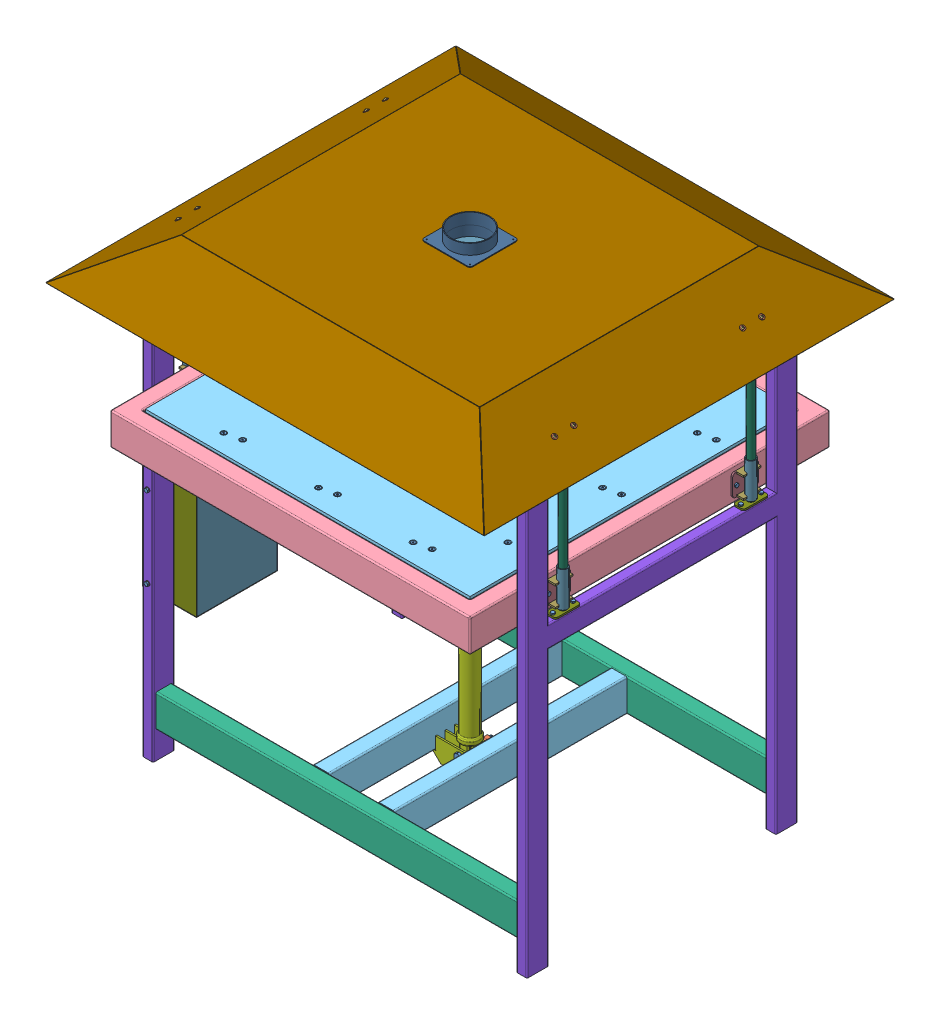
SolidWorks assembly SPR-V1 0000.00-A Sheetpress assembly, configuration Default. Lengths in mm. (continued)
Components (placement in the parent): (continued)
- Pressing plate lower^SPR-V1 0000.00-A Sheetpress assembly-1: Pressing plate lower^SPR-V1 0000.00-A Sheetpress assembly [Default] at origin size (1356.27 262 1540) (virtual) (continued)
  - socket countersunk head screw_iso-11: socket countersunk head screw_iso [ISO 10642 - M8 x 50 - 28N] at (378.5001 -297 168.4165) x (0 -1 0) z (-0.546944 0 0.837169) size (50 15.24 15.24)
  - socket countersunk head screw_iso-12: socket countersunk head screw_iso [ISO 10642 - M8 x 50 - 28N] at (553.502 -297 343.4183) x (0 -1 0) z (-0.546944 0 0.837169) size (50 15.24 15.24)
  - socket countersunk head screw_iso-13: socket countersunk head screw_iso [ISO 10642 - M8 x 50 - 28N] at (-496.5092 -297 -356.5891) x (0 -1 0) z (-0.546944 0 0.837169) size (50 15.24 15.24)
  - socket countersunk head screw_iso-14: socket countersunk head screw_iso [ISO 10642 - M8 x 50 - 28N] at (-321.5073 -297 -181.5872) x (0 -1 0) z (-0.546944 0 0.837169) size (50 15.24 15.24)
  - socket countersunk head screw_iso-15: socket countersunk head screw_iso [ISO 10642 - M8 x 50 - 28N] at (-146.5055 -297 -6.5854) x (0 -1 0) z (-0.546944 0 0.837169) size (50 15.24 15.24)
  - socket countersunk head screw_iso-16: socket countersunk head screw_iso [ISO 10642 - M8 x 50 - 28N] at (28.4964 -297 168.4165) x (0 -1 0) z (-0.546944 0 0.837169) size (50 15.24 15.24)
  - socket countersunk head screw_iso-17: socket countersunk head screw_iso [ISO 10642 - M8 x 50 - 28N] at (203.4983 -297 343.4183) x (0 -1 0) z (-0.546944 0 0.837169) size (50 15.24 15.24)
  - socket countersunk head screw_iso-18: socket countersunk head screw_iso [ISO 10642 - M8 x 50 - 28N] at (378.5001 -297 518.4202) x (0 -1 0) z (-0.546944 0 0.837169) size (50 15.24 15.24)
  - socket countersunk head screw_iso-19: socket countersunk head screw_iso [ISO 10642 - M8 x 50 - 28N] at (-496.5092 -297 -6.5854) x (0 -1 0) z (-0.546944 0 0.837169) size (50 15.24 15.24)
  - socket countersunk head screw_iso-20: socket countersunk head screw_iso [ISO 10642 - M8 x 50 - 28N] at (-321.5073 -297 168.4165) x (0 -1 0) z (-0.546944 0 0.837169) size (50 15.24 15.24)
  - socket countersunk head screw_iso-21: socket countersunk head screw_iso [ISO 10642 - M8 x 50 - 28N] at (-146.5055 -297 343.4183) x (0 -1 0) z (-0.546944 0 0.837169) size (50 15.24 15.24)
  - socket countersunk head screw_iso-22: socket countersunk head screw_iso [ISO 10642 - M8 x 50 - 28N] at (28.4964 -297 518.4202) x (0 -1 0) z (-0.546944 0 0.837169) size (50 15.24 15.24)
  - socket countersunk head screw_iso-23: socket countersunk head screw_iso [ISO 10642 - M8 x 50 - 28N] at (-496.5092 -297 343.4183) x (0 -1 0) z (-0.546944 0 0.837169) size (50 15.24 15.24)
  - socket countersunk head screw_iso-24: socket countersunk head screw_iso [ISO 10642 - M8 x 50 - 28N] at (-321.5073 -297 518.4202) x (0 -1 0) z (-0.546944 0 0.837169) size (50 15.24 15.24)
  - socket countersunk head screw_iso-25: socket countersunk head screw_iso [ISO 10642 - M8 x 50 - 28N] at (321.5073 -297 -518.4388) x (0 -1 0) z (-0.546944 0 0.837169) size (50 15.24 15.24)
  - socket countersunk head screw_iso-26: socket countersunk head screw_iso [ISO 10642 - M8 x 50 - 28N] at (496.5092 -297 -343.4369) x (0 -1 0) z (-0.546944 0 0.837169) size (50 15.24 15.24)
  - socket countersunk head screw_iso-27: socket countersunk head screw_iso [ISO 10642 - M8 x 50 - 28N] at (-28.4964 -297 -518.4388) x (0 -1 0) z (-0.546944 0 0.837169) size (50 15.24 15.24)
  - socket countersunk head screw_iso-28: socket countersunk head screw_iso [ISO 10642 - M8 x 50 - 28N] at (146.5055 -297 -343.4369) x (0 -1 0) z (-0.546944 0 0.837169) size (50 15.24 15.24)
  - socket countersunk head screw_iso-29: socket countersunk head screw_iso [ISO 10642 - M8 x 50 - 28N] at (321.5073 -297 -168.4351) x (0 -1 0) z (-0.546944 0 0.837169) size (50 15.24 15.24)
  - socket countersunk head screw_iso-30: socket countersunk head screw_iso [ISO 10642 - M8 x 50 - 28N] at (496.5092 -297 6.5668) x (0 -1 0) z (-0.546944 0 0.837169) size (50 15.24 15.24)
  - socket countersunk head screw_iso-31: socket countersunk head screw_iso [ISO 10642 - M8 x 50 - 28N] at (-378.5001 -297 -518.4388) x (0 -1 0) z (-0.546944 0 0.837169) size (50 15.24 15.24)
  - socket countersunk head screw_iso-32: socket countersunk head screw_iso [ISO 10642 - M8 x 50 - 28N] at (-203.4983 -297 -343.4369) x (0 -1 0) z (-0.546944 0 0.837169) size (50 15.24 15.24)
  - socket countersunk head screw_iso-33: socket countersunk head screw_iso [ISO 10642 - M8 x 50 - 28N] at (-28.4964 -297 -168.4351) x (0 -1 0) z (-0.546944 0 0.837169) size (50 15.24 15.24)
  - socket countersunk head screw_iso-34: socket countersunk head screw_iso [ISO 10642 - M8 x 50 - 28N] at (146.5055 -297 6.5668) x (0 -1 0) z (-0.546944 0 0.837169) size (50 15.24 15.24)
  - socket countersunk head screw_iso-35: socket countersunk head screw_iso [ISO 10642 - M8 x 50 - 28N] at (321.5073 -297 181.5687) x (0 -1 0) z (-0.546944 0 0.837169) size (50 15.24 15.24)
  - socket countersunk head screw_iso-36: socket countersunk head screw_iso [ISO 10642 - M8 x 50 - 28N] at (496.5092 -297 356.5705) x (0 -1 0) z (-0.546944 0 0.837169) size (50 15.24 15.24)
  - socket countersunk head screw_iso-37: socket countersunk head screw_iso [ISO 10642 - M8 x 50 - 28N] at (-553.502 -297 -343.4369) x (0 -1 0) z (-0.546944 0 0.837169) size (50 15.24 15.24)
  - socket countersunk head screw_iso-38: socket countersunk head screw_iso [ISO 10642 - M8 x 50 - 28N] at (-378.5001 -297 -168.4351) x (0 -1 0) z (-0.546944 0 0.837169) size (50 15.24 15.24)
  - socket countersunk head screw_iso-39: socket countersunk head screw_iso [ISO 10642 - M8 x 50 - 28N] at (-203.4983 -297 6.5668) x (0 -1 0) z (-0.546944 0 0.837169) size (50 15.24 15.24)
  - socket countersunk head screw_iso-40: socket countersunk head screw_iso [ISO 10642 - M8 x 50 - 28N] at (-28.4964 -297 181.5687) x (0 -1 0) z (-0.546944 0 0.837169) size (50 15.24 15.24)
  - socket countersunk head screw_iso-41: socket countersunk head screw_iso [ISO 10642 - M8 x 50 - 28N] at (146.5055 -297 356.5705) x (0 -1 0) z (-0.546944 0 0.837169) size (50 15.24 15.24)
  - socket countersunk head screw_iso-42: socket countersunk head screw_iso [ISO 10642 - M8 x 50 - 28N] at (321.5073 -297 531.5724) x (0 -1 0) z (-0.546944 0 0.837169) size (50 15.24 15.24)
  - socket countersunk head screw_iso-43: socket countersunk head screw_iso [ISO 10642 - M8 x 50 - 28N] at (-553.502 -297 6.5668) x (0 -1 0) z (-0.546944 0 0.837169) size (50 15.24 15.24)
  - socket countersunk head screw_iso-44: socket countersunk head screw_iso [ISO 10642 - M8 x 50 - 28N] at (-378.5001 -297 181.5687) x (0 -1 0) z (-0.546944 0 0.837169) size (50 15.24 15.24)
  - socket countersunk head screw_iso-45: socket countersunk head screw_iso [ISO 10642 - M8 x 50 - 28N] at (-203.4983 -297 356.5705) x (0 -1 0) z (-0.546944 0 0.837169) size (50 15.24 15.24)
  - socket countersunk head screw_iso-46: socket countersunk head screw_iso [ISO 10642 - M8 x 50 - 28N] at (-28.4964 -297 531.5724) x (0 -1 0) z (-0.546944 0 0.837169) size (50 15.24 15.24)
  - socket countersunk head screw_iso-47: socket countersunk head screw_iso [ISO 10642 - M8 x 50 - 28N] at (-553.502 -297 356.5705) x (0 -1 0) z (-0.546944 0 0.837169) size (50 15.24 15.24)
  - socket countersunk head screw_iso-48: socket countersunk head screw_iso [ISO 10642 - M8 x 50 - 28N] at (-378.5001 -297 531.5724) x (0 -1 0) z (-0.546944 0 0.837169) size (50 15.24 15.24)
  - plain washer normal grade a_iso-1: plain washer normal grade a_iso [Washer ISO 7089 - 8] at (378.5001 -333.6 -531.591) x (0 -1 0) z (0 0 1) size (1.6 16 16)
  - plain washer normal grade a_iso-2: plain washer normal grade a_iso [Washer ISO 7089 - 8] at (553.502 -333.6 -356.5891) x (0 -1 0) z (0 0 1) size (1.6 16 16)
  - plain washer normal grade a_iso-3: plain washer normal grade a_iso [Washer ISO 7089 - 8] at (28.4964 -333.6 -531.591) x (0 -1 0) z (0 0 1) size (1.6 16 16)
  - plain washer normal grade a_iso-4: plain washer normal grade a_iso [Washer ISO 7089 - 8] at (203.4983 -333.6 -356.5891) x (0 -1 0) z (0 0 1) size (1.6 16 16)
  - plain washer normal grade a_iso-5: plain washer normal grade a_iso [Washer ISO 7089 - 8] at (378.5001 -333.6 -181.5872) x (0 -1 0) z (0 0 1) size (1.6 16 16)
  - plain washer normal grade a_iso-6: plain washer normal grade a_iso [Washer ISO 7089 - 8] at (553.502 -333.6 -6.5854) x (0 -1 0) z (0 0 1) size (1.6 16 16)
  - plain washer normal grade a_iso-7: plain washer normal grade a_iso [Washer ISO 7089 - 8] at (-321.5073 -333.6 -531.591) x (0 -1 0) z (0 0 1) size (1.6 16 16)
  - plain washer normal grade a_iso-8: plain washer normal grade a_iso [Washer ISO 7089 - 8] at (-146.5055 -333.6 -356.5891) x (0 -1 0) z (0 0 1) size (1.6 16 16)
  - plain washer normal grade a_iso-9: plain washer normal grade a_iso [Washer ISO 7089 - 8] at (28.4964 -333.6 -181.5872) x (0 -1 0) z (0 0 1) size (1.6 16 16)
  - plain washer normal grade a_iso-10: plain washer normal grade a_iso [Washer ISO 7089 - 8] at (203.4983 -333.6 -6.5854) x (0 -1 0) z (0 0 1) size (1.6 16 16)
  - plain washer normal grade a_iso-11: plain washer normal grade a_iso [Washer ISO 7089 - 8] at (378.5001 -333.6 168.4165) x (0 -1 0) z (0 0 1) size (1.6 16 16)
  - plain washer normal grade a_iso-12: plain washer normal grade a_iso [Washer ISO 7089 - 8] at (553.502 -333.6 343.4183) x (0 -1 0) z (0 0 1) size (1.6 16 16)
  - plain washer normal grade a_iso-13: plain washer normal grade a_iso [Washer ISO 7089 - 8] at (-496.5092 -333.6 -356.5891) x (0 -1 0) z (0 0 1) size (1.6 16 16)
  - plain washer normal grade a_iso-14: plain washer normal grade a_iso [Washer ISO 7089 - 8] at (-321.5073 -333.6 -181.5872) x (0 -1 0) z (0 0 1) size (1.6 16 16)
  - plain washer normal grade a_iso-15: plain washer normal grade a_iso [Washer ISO 7089 - 8] at (-146.5055 -333.6 -6.5854) x (0 -1 0) z (0 0 1) size (1.6 16 16)
  - plain washer normal grade a_iso-16: plain washer normal grade a_iso [Washer ISO 7089 - 8] at (28.4964 -333.6 168.4165) x (0 -1 0) z (0 0 1) size (1.6 16 16)
  - plain washer normal grade a_iso-17: plain washer normal grade a_iso [Washer ISO 7089 - 8] at (203.4983 -333.6 343.4183) x (0 -1 0) z (0 0 1) size (1.6 16 16)
  - plain washer normal grade a_iso-18: plain washer normal grade a_iso [Washer ISO 7089 - 8] at (378.5001 -333.6 518.4202) x (0 -1 0) z (0 0 1) size (1.6 16 16)
  - plain washer normal grade a_iso-19: plain washer normal grade a_iso [Washer ISO 7089 - 8] at (-496.5092 -333.6 -6.5854) x (0 -1 0) z (0 0 1) size (1.6 16 16)
  - plain washer normal grade a_iso-20: plain washer normal grade a_iso [Washer ISO 7089 - 8] at (-321.5073 -333.6 168.4165) x (0 -1 0) z (0 0 1) size (1.6 16 16)
  - plain washer normal grade a_iso-21: plain washer normal grade a_iso [Washer ISO 7089 - 8] at (-146.5055 -333.6 343.4183) x (0 -1 0) z (0 0 1) size (1.6 16 16)
  - plain washer normal grade a_iso-22: plain washer normal grade a_iso [Washer ISO 7089 - 8] at (28.4964 -333.6 518.4202) x (0 -1 0) z (0 0 1) size (1.6 16 16)
  - plain washer normal grade a_iso-23: plain washer normal grade a_iso [Washer ISO 7089 - 8] at (-496.5092 -333.6 343.4183) x (0 -1 0) z (0 0 1) size (1.6 16 16)
  - plain washer normal grade a_iso-24: plain washer normal grade a_iso [Washer ISO 7089 - 8] at (-321.5073 -333.6 518.4202) x (0 -1 0) z (0 0 1) size (1.6 16 16)
  - plain washer normal grade a_iso-25: plain washer normal grade a_iso [Washer ISO 7089 - 8] at (321.5073 -332 -518.4388) x (0 1 0) z (0 0 1) size (1.6 16 16)
  - plain washer normal grade a_iso-26: plain washer normal grade a_iso [Washer ISO 7089 - 8] at (496.5092 -332 -343.4369) x (0 1 0) z (0 0 1) size (1.6 16 16)
  - plain washer normal grade a_iso-27: plain washer normal grade a_iso [Washer ISO 7089 - 8] at (-28.4964 -332 -518.4388) x (0 1 0) z (0 0 1) size (1.6 16 16)
  - plain washer normal grade a_iso-28: plain washer normal grade a_iso [Washer ISO 7089 - 8] at (146.5055 -332 -343.4369) x (0 1 0) z (0 0 1) size (1.6 16 16)
  - plain washer normal grade a_iso-29: plain washer normal grade a_iso [Washer ISO 7089 - 8] at (321.5073 -332 -168.4351) x (0 1 0) z (0 0 1) size (1.6 16 16)
  - plain washer normal grade a_iso-30: plain washer normal grade a_iso [Washer ISO 7089 - 8] at (496.5092 -332 6.5668) x (0 1 0) z (0 0 1) size (1.6 16 16)
  - plain washer normal grade a_iso-31: plain washer normal grade a_iso [Washer ISO 7089 - 8] at (-378.5001 -332 -518.4388) x (0 1 0) z (0 0 1) size (1.6 16 16)
  - plain washer normal grade a_iso-32: plain washer normal grade a_iso [Washer ISO 7089 - 8] at (-203.4983 -332 -343.4369) x (0 1 0) z (0 0 1) size (1.6 16 16)
  - plain washer normal grade a_iso-33: plain washer normal grade a_iso [Washer ISO 7089 - 8] at (-28.4964 -332 -168.4351) x (0 1 0) z (0 0 1) size (1.6 16 16)
  - plain washer normal grade a_iso-34: plain washer normal grade a_iso [Washer ISO 7089 - 8] at (146.5055 -332 6.5668) x (0 1 0) z (0 0 1) size (1.6 16 16)
  - plain washer normal grade a_iso-35: plain washer normal grade a_iso [Washer ISO 7089 - 8] at (321.5073 -332 181.5687) x (0 1 0) z (0 0 1) size (1.6 16 16)
  - plain washer normal grade a_iso-36: plain washer normal grade a_iso [Washer ISO 7089 - 8] at (496.5092 -332 356.5705) x (0 1 0) z (0 0 1) size (1.6 16 16)
  - plain washer normal grade a_iso-37: plain washer normal grade a_iso [Washer ISO 7089 - 8] at (-553.502 -332 -343.4369) x (0 1 0) z (0 0 1) size (1.6 16 16)
  - plain washer normal grade a_iso-38: plain washer normal grade a_iso [Washer ISO 7089 - 8] at (-378.5001 -332 -168.4351) x (0 1 0) z (0 0 1) size (1.6 16 16)
  - plain washer normal grade a_iso-39: plain washer normal grade a_iso [Washer ISO 7089 - 8] at (-203.4983 -332 6.5668) x (0 1 0) z (0 0 1) size (1.6 16 16)
  - plain washer normal grade a_iso-40: plain washer normal grade a_iso [Washer ISO 7089 - 8] at (-28.4964 -332 181.5687) x (0 1 0) z (0 0 1) size (1.6 16 16)
  - plain washer normal grade a_iso-41: plain washer normal grade a_iso [Washer ISO 7089 - 8] at (146.5055 -332 356.5705) x (0 1 0) z (0 0 1) size (1.6 16 16)
  - plain washer normal grade a_iso-42: plain washer normal grade a_iso [Washer ISO 7089 - 8] at (321.5073 -332 531.5724) x (0 1 0) z (0 0 1) size (1.6 16 16)
  - plain washer normal grade a_iso-43: plain washer normal grade a_iso [Washer ISO 7089 - 8] at (-553.502 -332 6.5668) x (0 1 0) z (0 0 1) size (1.6 16 16)
  - plain washer normal grade a_iso-44: plain washer normal grade a_iso [Washer ISO 7089 - 8] at (-378.5001 -332 181.5687) x (0 1 0) z (0 0 1) size (1.6 16 16)
  - plain washer normal grade a_iso-45: plain washer normal grade a_iso [Washer ISO 7089 - 8] at (-203.4983 -332 356.5705) x (0 1 0) z (0 0 1) size (1.6 16 16)
  - plain washer normal grade a_iso-46: plain washer normal grade a_iso [Washer ISO 7089 - 8] at (-28.4964 -332 531.5724) x (0 1 0) z (0 0 1) size (1.6 16 16)
  - plain washer normal grade a_iso-47: plain washer normal grade a_iso [Washer ISO 7089 - 8] at (-553.502 -332 356.5705) x (0 1 0) z (0 0 1) size (1.6 16 16)
  - plain washer normal grade a_iso-48: plain washer normal grade a_iso [Washer ISO 7089 - 8] at (-378.5001 -332 531.5724) x (0 1 0) z (0 0 1) size (1.6 16 16)
  - hex nut gradec_iso-1: hex nut gradec_iso [ISO - 4034 - M8 - N] at (378.5001 -341.5 -531.591) x (1 0 0) z (0 -1 0) size (13 15.01 7.9)
  - hex nut gradec_iso-2: hex nut gradec_iso [ISO - 4034 - M8 - N] at (553.502 -341.5 -356.5891) x (1 0 0) z (0 -1 0) size (13 15.01 7.9)
  - hex nut gradec_iso-3: hex nut gradec_iso [ISO - 4034 - M8 - N] at (28.4964 -341.5 -531.591) x (1 0 0) z (0 -1 0) size (13 15.01 7.9)
  - hex nut gradec_iso-4: hex nut gradec_iso [ISO - 4034 - M8 - N] at (203.4983 -341.5 -356.5891) x (1 0 0) z (0 -1 0) size (13 15.01 7.9)
  - hex nut gradec_iso-5: hex nut gradec_iso [ISO - 4034 - M8 - N] at (378.5001 -341.5 -181.5872) x (1 0 0) z (0 -1 0) size (13 15.01 7.9)
  - hex nut gradec_iso-6: hex nut gradec_iso [ISO - 4034 - M8 - N] at (553.502 -341.5 -6.5854) x (1 0 0) z (0 -1 0) size (13 15.01 7.9)
  - hex nut gradec_iso-7: hex nut gradec_iso [ISO - 4034 - M8 - N] at (-321.5073 -341.5 -531.591) x (1 0 0) z (0 -1 0) size (13 15.01 7.9)
  - hex nut gradec_iso-8: hex nut gradec_iso [ISO - 4034 - M8 - N] at (-146.5055 -341.5 -356.5891) x (1 0 0) z (0 -1 0) size (13 15.01 7.9)
  - hex nut gradec_iso-9: hex nut gradec_iso [ISO - 4034 - M8 - N] at (28.4964 -341.5 -181.5872) x (1 0 0) z (0 -1 0) size (13 15.01 7.9)
  - hex nut gradec_iso-10: hex nut gradec_iso [ISO - 4034 - M8 - N] at (203.4983 -341.5 -6.5854) x (1 0 0) z (0 -1 0) size (13 15.01 7.9)
  - hex nut gradec_iso-11: hex nut gradec_iso [ISO - 4034 - M8 - N] at (378.5001 -341.5 168.4165) x (1 0 0) z (0 -1 0) size (13 15.01 7.9)
  - hex nut gradec_iso-12: hex nut gradec_iso [ISO - 4034 - M8 - N] at (553.502 -341.5 343.4183) x (1 0 0) z (0 -1 0) size (13 15.01 7.9)
  - hex nut gradec_iso-13: hex nut gradec_iso [ISO - 4034 - M8 - N] at (-496.5092 -341.5 -356.5891) x (1 0 0) z (0 -1 0) size (13 15.01 7.9)
  - hex nut gradec_iso-14: hex nut gradec_iso [ISO - 4034 - M8 - N] at (-321.5073 -341.5 -181.5872) x (1 0 0) z (0 -1 0) size (13 15.01 7.9)
  - hex nut gradec_iso-15: hex nut gradec_iso [ISO - 4034 - M8 - N] at (-146.5055 -341.5 -6.5854) x (1 0 0) z (0 -1 0) size (13 15.01 7.9)
  - hex nut gradec_iso-16: hex nut gradec_iso [ISO - 4034 - M8 - N] at (28.4964 -341.5 168.4165) x (1 0 0) z (0 -1 0) size (13 15.01 7.9)
  - hex nut gradec_iso-17: hex nut gradec_iso [ISO - 4034 - M8 - N] at (203.4983 -341.5 343.4183) x (1 0 0) z (0 -1 0) size (13 15.01 7.9)
  - hex nut gradec_iso-18: hex nut gradec_iso [ISO - 4034 - M8 - N] at (378.5001 -341.5 518.4202) x (1 0 0) z (0 -1 0) size (13 15.01 7.9)
  - hex nut gradec_iso-19: hex nut gradec_iso [ISO - 4034 - M8 - N] at (-496.5092 -341.5 -6.5854) x (1 0 0) z (0 -1 0) size (13 15.01 7.9)
  - hex nut gradec_iso-20: hex nut gradec_iso [ISO - 4034 - M8 - N] at (-321.5073 -341.5 168.4165) x (1 0 0) z (0 -1 0) size (13 15.01 7.9)
  - hex nut gradec_iso-21: hex nut gradec_iso [ISO - 4034 - M8 - N] at (-146.5055 -341.5 343.4183) x (1 0 0) z (0 -1 0) size (13 15.01 7.9)
  - hex nut gradec_iso-22: hex nut gradec_iso [ISO - 4034 - M8 - N] at (28.4964 -341.5 518.4202) x (1 0 0) z (0 -1 0) size (13 15.01 7.9)
  - hex nut gradec_iso-23: hex nut gradec_iso [ISO - 4034 - M8 - N] at (-496.5092 -341.5 343.4183) x (1 0 0) z (0 -1 0) size (13 15.01 7.9)
  - hex nut gradec_iso-24: hex nut gradec_iso [ISO - 4034 - M8 - N] at (-321.5073 -341.5 518.4202) x (1 0 0) z (0 -1 0) size (13 15.01 7.9)
  - hex nut gradec_iso-25: hex nut gradec_iso [ISO - 4034 - M8 - N] at (321.5073 -341.5 -518.4388) x (1 0 0) z (0 -1 0) size (13 15.01 7.9)
  - hex nut gradec_iso-26: hex nut gradec_iso [ISO - 4034 - M8 - N] at (496.5092 -341.5 -343.4369) x (1 0 0) z (0 -1 0) size (13 15.01 7.9)
  - hex nut gradec_iso-27: hex nut gradec_iso [ISO - 4034 - M8 - N] at (-28.4964 -341.5 -518.4388) x (1 0 0) z (0 -1 0) size (13 15.01 7.9)
  - hex nut gradec_iso-28: hex nut gradec_iso [ISO - 4034 - M8 - N] at (146.5055 -341.5 -343.4369) x (1 0 0) z (0 -1 0) size (13 15.01 7.9)
  - hex nut gradec_iso-29: hex nut gradec_iso [ISO - 4034 - M8 - N] at (321.5073 -341.5 -168.4351) x (1 0 0) z (0 -1 0) size (13 15.01 7.9)
  - hex nut gradec_iso-30: hex nut gradec_iso [ISO - 4034 - M8 - N] at (496.5092 -341.5 6.5668) x (1 0 0) z (0 -1 0) size (13 15.01 7.9)
  - hex nut gradec_iso-31: hex nut gradec_iso [ISO - 4034 - M8 - N] at (-378.5001 -341.5 -518.4388) x (1 0 0) z (0 -1 0) size (13 15.01 7.9)
  - hex nut gradec_iso-32: hex nut gradec_iso [ISO - 4034 - M8 - N] at (-203.4983 -341.5 -343.4369) x (1 0 0) z (0 -1 0) size (13 15.01 7.9)
  - hex nut gradec_iso-33: hex nut gradec_iso [ISO - 4034 - M8 - N] at (-28.4964 -341.5 -168.4351) x (1 0 0) z (0 -1 0) size (13 15.01 7.9)
  - hex nut gradec_iso-34: hex nut gradec_iso [ISO - 4034 - M8 - N] at (146.5055 -341.5 6.5668) x (1 0 0) z (0 -1 0) size (13 15.01 7.9)
  - hex nut gradec_iso-35: hex nut gradec_iso [ISO - 4034 - M8 - N] at (321.5073 -341.5 181.5687) x (1 0 0) z (0 -1 0) size (13 15.01 7.9)
  - hex nut gradec_iso-36: hex nut gradec_iso [ISO - 4034 - M8 - N] at (496.5092 -341.5 356.5705) x (1 0 0) z (0 -1 0) size (13 15.01 7.9)
  - hex nut gradec_iso-37: hex nut gradec_iso [ISO - 4034 - M8 - N] at (-553.502 -341.5 -343.4369) x (1 0 0) z (0 -1 0) size (13 15.01 7.9)
  - hex nut gradec_iso-38: hex nut gradec_iso [ISO - 4034 - M8 - N] at (-378.5001 -341.5 -168.4351) x (1 0 0) z (0 -1 0) size (13 15.01 7.9)
  - hex nut gradec_iso-39: hex nut gradec_iso [ISO - 4034 - M8 - N] at (-203.4983 -341.5 6.5668) x (1 0 0) z (0 -1 0) size (13 15.01 7.9)
  - hex nut gradec_iso-40: hex nut gradec_iso [ISO - 4034 - M8 - N] at (-28.4964 -341.5 181.5687) x (1 0 0) z (0 -1 0) size (13 15.01 7.9)
  - hex nut gradec_iso-41: hex nut gradec_iso [ISO - 4034 - M8 - N] at (146.5055 -341.5 356.5705) x (1 0 0) z (0 -1 0) size (13 15.01 7.9)
  - hex nut gradec_iso-42: hex nut gradec_iso [ISO - 4034 - M8 - N] at (321.5073 -341.5 531.5724) x (1 0 0) z (0 -1 0) size (13 15.01 7.9)
  - hex nut gradec_iso-43: hex nut gradec_iso [ISO - 4034 - M8 - N] at (-553.502 -341.5 6.5668) x (1 0 0) z (0 -1 0) size (13 15.01 7.9)
  - hex nut gradec_iso-44: hex nut gradec_iso [ISO - 4034 - M8 - N] at (-378.5001 -341.5 181.5687) x (1 0 0) z (0 -1 0) size (13 15.01 7.9)
  - hex nut gradec_iso-45: hex nut gradec_iso [ISO - 4034 - M8 - N] at (-203.4983 -341.5 356.5705) x (1 0 0) z (0 -1 0) size (13 15.01 7.9)
  - hex nut gradec_iso-46: hex nut gradec_iso [ISO - 4034 - M8 - N] at (-28.4964 -341.5 531.5724) x (1 0 0) z (0 -1 0) size (13 15.01 7.9)
  - hex nut gradec_iso-47: hex nut gradec_iso [ISO - 4034 - M8 - N] at (-553.502 -341.5 356.5705) x (1 0 0) z (0 -1 0) size (13 15.01 7.9)
  - hex nut gradec_iso-48: hex nut gradec_iso [ISO - 4034 - M8 - N] at (-378.5001 -341.5 531.5724) x (1 0 0) z (0 -1 0) size (13 15.01 7.9)
  - socket countersunk head screw_iso-49: socket countersunk head screw_iso [ISO 10642 - M8 x 50 - 28N] at (-246.2365 -297 278.7635) x (0 -1 0) z (1 0 0) size (50 15.24 15.24)
  - socket countersunk head screw_iso-50: socket countersunk head screw_iso [ISO 10642 - M8 x 50 - 28N] at (-278.7635 -297 -246.2365) x (0 -1 0) z (0 0 1) size (50 15.24 15.24)
  - socket countersunk head screw_iso-51: socket countersunk head screw_iso [ISO 10642 - M8 x 50 - 28N] at (246.2365 -297 -278.7635) x (0 -1 0) z (-1 0 0) size (50 15.24 15.24)
  - socket countersunk head screw_iso-52: socket countersunk head screw_iso [ISO 10642 - M8 x 50 - 28N] at (278.7635 -297 246.2365) x (0 -1 0) z (0 0 -1) size (50 15.24 15.24)
  - socket countersunk head screw_iso-53: socket countersunk head screw_iso [ISO 10642 - M8 x 50 - 28N] at (-278.7635 -297 246.2365) x (0 -1 0) z (1 0 0) size (50 15.24 15.24)
  - socket countersunk head screw_iso-54: socket countersunk head screw_iso [ISO 10642 - M8 x 50 - 28N] at (-246.2365 -297 -278.7635) x (0 -1 0) z (0 0 1) size (50 15.24 15.24)
  - socket countersunk head screw_iso-55: socket countersunk head screw_iso [ISO 10642 - M8 x 50 - 28N] at (278.7635 -297 -246.2365) x (0 -1 0) z (-1 0 0) size (50 15.24 15.24)
  - socket countersunk head screw_iso-56: socket countersunk head screw_iso [ISO 10642 - M8 x 50 - 28N] at (246.2365 -297 278.7635) x (0 -1 0) z (0 0 -1) size (50 15.24 15.24)
  - hex nut gradec_iso-49: hex nut gradec_iso [ISO - 4034 - M8 - N] at (246.2365 -339.9 -278.7635) x (1 0 0) z (0 -1 0) size (13 15.01 7.9)
  - hex nut gradec_iso-50: hex nut gradec_iso [ISO - 4034 - M8 - N] at (278.7635 -339.9 -246.2365) x (1 0 0) z (0 -1 0) size (13 15.01 7.9)
  - hex nut gradec_iso-51: hex nut gradec_iso [ISO - 4034 - M8 - N] at (278.7635 -339.9 246.2365) x (1 0 0) z (0 -1 0) size (13 15.01 7.9)
  - hex nut gradec_iso-52: hex nut gradec_iso [ISO - 4034 - M8 - N] at (246.2365 -339.9 278.7635) x (1 0 0) z (0 -1 0) size (13 15.01 7.9)
  - hex nut gradec_iso-53: hex nut gradec_iso [ISO - 4034 - M8 - N] at (-278.7635 -339.9 246.2365) x (1 0 0) z (0 -1 0) size (13 15.01 7.9)
  - hex nut gradec_iso-54: hex nut gradec_iso [ISO - 4034 - M8 - N] at (-246.2365 -339.9 278.7635) x (1 0 0) z (0 -1 0) size (13 15.01 7.9)
  - hex nut gradec_iso-55: hex nut gradec_iso [ISO - 4034 - M8 - N] at (-278.7635 -339.9 -246.2365) x (1 0 0) z (0 -1 0) size (13 15.01 7.9)
  - hex nut gradec_iso-56: hex nut gradec_iso [ISO - 4034 - M8 - N] at (-246.2365 -339.9 -278.7635) x (1 0 0) z (0 -1 0) size (13 15.01 7.9)
  - plain washer large grade ac_iso-1: plain washer large grade ac_iso [Washer ISO 7093 - 6] at (-525 -419.5 -585) x (0 1 0) z (0 0 1) size (1.6 18 18)
  - plain washer large grade ac_iso-2: plain washer large grade ac_iso [Washer ISO 7093 - 6] at (-585 -419.5 -525) x (0 1 0) z (0 0 1) size (1.6 18 18)
  - plain washer large grade ac_iso-3: plain washer large grade ac_iso [Washer ISO 7093 - 6] at (0 -419.5 -29.2426) x (0 1 0) z (0 0 1) size (1.6 18 18)
  - plain washer large grade ac_iso-4: plain washer large grade ac_iso [Washer ISO 7093 - 6] at (29.2426 -419.5 0) x (0 1 0) z (0 0 1) size (1.6 18 18)
  - plain washer large grade ac_iso-5: plain washer large grade ac_iso [Washer ISO 7093 - 6] at (525 -419.5 -585) x (0 1 0) z (0 0 1) size (1.6 18 18)
  - plain washer large grade ac_iso-6: plain washer large grade ac_iso [Washer ISO 7093 - 6] at (585 -419.5 -525) x (0 1 0) z (0 0 1) size (1.6 18 18)
  - plain washer large grade ac_iso-7: plain washer large grade ac_iso [Washer ISO 7093 - 6] at (585 -419.5 525) x (0 1 0) z (0 0 1) size (1.6 18 18)
  - plain washer large grade ac_iso-8: plain washer large grade ac_iso [Washer ISO 7093 - 6] at (525 -419.5 585) x (0 1 0) z (0 0 1) size (1.6 18 18)
  - plain washer large grade ac_iso-9: plain washer large grade ac_iso [Washer ISO 7093 - 6] at (-525 -419.5 585) x (0 1 0) z (0 0 1) size (1.6 18 18)
  - plain washer large grade ac_iso-10: plain washer large grade ac_iso [Washer ISO 7093 - 6] at (-585 -419.5 525) x (0 1 0) z (0 0 1) size (1.6 18 18)
  - plain washer large grade ac_iso-11: plain washer large grade ac_iso [Washer ISO 7093 - 6] at (0 -419.5 29.2426) x (0 1 0) z (0 0 1) size (1.6 18 18)
  - socket button head screw_iso-1: socket button head screw_iso [ISO 7380 - M6 x 12 - 12N] at (-585 -424.4 -525) x (0 1 0) z (0 0 1) size (15.3 10.5 10.5)
  - socket button head screw_iso-2: socket button head screw_iso [ISO 7380 - M6 x 12 - 12N] at (-525 -424.4 -585) x (0 1 0) z (0 0 1) size (15.3 10.5 10.5)
  - socket button head screw_iso-3: socket button head screw_iso [ISO 7380 - M6 x 12 - 12N] at (-29.2426 -424.4 0) x (0 1 0) z (0 0 1) size (15.3 10.5 10.5)
  - socket button head screw_iso-4: socket button head screw_iso [ISO 7380 - M6 x 12 - 12N] at (0 -424.4 -29.2426) x (0 1 0) z (0 0 1) size (15.3 10.5 10.5)
  - socket button head screw_iso-5: socket button head screw_iso [ISO 7380 - M6 x 12 - 12N] at (585 -424.4 525) x (0 1 0) z (0 0 1) size (15.3 10.5 10.5)
  - socket button head screw_iso-6: socket button head screw_iso [ISO 7380 - M6 x 12 - 12N] at (525 -424.4 585) x (0 1 0) z (0 0 1) size (15.3 10.5 10.5)
  - socket button head screw_iso-7: socket button head screw_iso [ISO 7380 - M6 x 12 - 12N] at (29.2426 -424.4 0) x (0 1 0) z (0 0 1) size (15.3 10.5 10.5)
  - socket button head screw_iso-8: socket button head screw_iso [ISO 7380 - M6 x 12 - 12N] at (0 -424.4 29.2426) x (0 1 0) z (0 0 1) size (15.3 10.5 10.5)
  - socket button head screw_iso-9: socket button head screw_iso [ISO 7380 - M6 x 12 - 12N] at (-525 -424.4 585) x (0 1 0) z (0 0 1) size (15.3 10.5 10.5)
  - socket button head screw_iso-10: socket button head screw_iso [ISO 7380 - M6 x 12 - 12N] at (-585 -424.4 525) x (0 1 0) z (0 0 1) size (15.3 10.5 10.5)
  - socket button head screw_iso-11: socket button head screw_iso [ISO 7380 - M6 x 12 - 12N] at (585 -424.4 -525) x (0 1 0) z (0 0 1) size (15.3 10.5 10.5)
  - socket button head screw_iso-12: socket button head screw_iso [ISO 7380 - M6 x 12 - 12N] at (525 -424.4 -585) x (0 1 0) z (0 0 1) size (15.3 10.5 10.5)
  - plain washer large grade ac_iso-12: plain washer large grade ac_iso [Washer ISO 7093 - 6] at (-29.2426 -419.5 0) x (0 1 0) z (0 0 1) size (1.6 18 18)
- Sliding mechanism^SPR-V1 0000.00-A Sheetpress assembly-1: Sliding mechanism^SPR-V1 0000.00-A Sheetpress assembly [Default] at origin size (1428.35 678.14 790) (virtual)
  - SPR-V1 1000.02-A Guide bracket-1: SPR-V1 1000.02-A Guide bracket [Default] at (665 -300 0) x (0 0 1) z (1 0 0) size (65 80 31)
  - SPR-V1 1000.02-A Guide plate-1: SPR-V1 1000.02-A Guide plate [Default] at (665 -300 0) x (0 0 1) z (1 0 0) size (95 80 6)
  - SPR-V1 1000.02-A Slider guide-1: SPR-V1 1000.02-A Slider guide [Default] at (665 -320 0) x (0 0 -1) z (0 1 0) size (34 34 130)
  - SPR-V1 1000.03-A Slider rod-1: SPR-V1 1000.03-A Slider rod [Default] at (671 -420 0) x (0 0 -1) z (0 1 0) size (27 27 460)
  - SPR-V1 1000.04-A Slider rod plate-1: SPR-V1 1000.04-A Slider rod plate [Default] at (671 -420 0) x (0 0 -1) z (0 1 0) size (95 40 6)
  - SPR-V1 1000.05-A Hood bracket 1-1: SPR-V1 1000.05-A Hood bracket 1 [Default] at (0 120 0) x (1 0 0) z (0 1 0) size (40 95 6)
  - SPR-V1 1000.05-A Hood bracket 2-1: SPR-V1 1000.05-A Hood bracket 2 [Default] at (0 0 -347.5) size (40 44.14 6)
  - SPR-V1 1000.05-A Hood bracket 3-1: SPR-V1 1000.05-A Hood bracket 3 [Default] at (0 0 -347.5) size (44.82 31.06 95)
  - SPR-V1 1000.02-A Slider guide-2: SPR-V1 1000.02-A Slider guide [Default] at (665 -370 0) x (0 0 1) z (0 -1 0) size (34 34 130)
  - SPR-V1 1000.03-A Slider rod-2: SPR-V1 1000.03-A Slider rod [Default] at (671 40 0) x (0 0 1) z (0 -1 0) size (27 27 460)
  - SPR-V1 1000.02-A Guide bracket-2: SPR-V1 1000.02-A Guide bracket [Default] at (665 -300 695) x (0 0 1) z (1 0 0) size (65 80 31)
  - SPR-V1 1000.02-A Slider guide-3: SPR-V1 1000.02-A Slider guide [Default] at (-665 -370 0) x (0 0 -1) z (0 -1 0) size (34 34 130)
  - SPR-V1 1000.03-A Slider rod-3: SPR-V1 1000.03-A Slider rod [Default] at (-671 40 0) x (0 0 -1) z (0 -1 0) size (27 27 460)
  - SPR-V1 1000.02-A Guide bracket-3: SPR-V1 1000.02-A Guide bracket [Default] at (-665 -300 -695) x (0 0 -1) z (-1 0 0) size (65 80 31)
  - SPR-V1 1000.02-A Slider guide-4: SPR-V1 1000.02-A Slider guide [Default] at (-665 -320 0) x (0 0 1) z (0 1 0) size (34 34 130)
  - SPR-V1 1000.03-A Slider rod-4: SPR-V1 1000.03-A Slider rod [Default] at (-671 -420 0) x (0 0 1) z (0 1 0) size (27 27 460)
  - SPR-V1 1000.02-A Guide bracket-4: SPR-V1 1000.02-A Guide bracket [Default] at (-665 -300 0) x (0 0 -1) z (-1 0 0) size (65 80 31)
  - SPR-V1 1000.02-A Guide plate-2: SPR-V1 1000.02-A Guide plate [Default] at (671 -300 0) x (0 0 -1) z (-1 0 0) size (95 80 6)
  - SPR-V1 1000.02-A Guide plate-3: SPR-V1 1000.02-A Guide plate [Default] at (-665 -300 0) x (0 0 -1) z (-1 0 0) size (95 80 6)
  - SPR-V1 1000.02-A Guide plate-4: SPR-V1 1000.02-A Guide plate [Default] at (-671 -300 0) x (0 0 1) z (1 0 0) size (95 80 6)
  - SPR-V1 1000.04-A Slider rod plate-2: SPR-V1 1000.04-A Slider rod plate [Default] at (671 -414 0) x (0 0 1) z (0 -1 0) size (95 40 6)
  - SPR-V1 1000.04-A Slider rod plate-3: SPR-V1 1000.04-A Slider rod plate [Default] at (-671 -414 0) x (0 0 -1) z (0 -1 0) size (95 40 6)
  - SPR-V1 1000.04-A Slider rod plate-4: SPR-V1 1000.04-A Slider rod plate [Default] at (-671 -420 0) x (0 0 1) z (0 1 0) size (95 40 6)
  - SPR-V1 1000.04-A Slider rod plate-5: SPR-V1 1000.04-A Slider rod plate [Default] at (671 40 0) x (0 0 1) z (0 -1 0) size (95 40 6)
  - SPR-V1 1000.04-A Slider rod plate-6: SPR-V1 1000.04-A Slider rod plate [Default] at (671 34 0) x (0 0 -1) z (0 1 0) size (95 40 6)
  - SPR-V1 1000.04-A Slider rod plate-7: SPR-V1 1000.04-A Slider rod plate [Default] at (-671 40 0) x (0 0 -1) z (0 -1 0) size (95 40 6)
  - SPR-V1 1000.04-A Slider rod plate-8: SPR-V1 1000.04-A Slider rod plate [Default] at (-671 34 0) x (0 0 1) z (0 1 0) size (95 40 6)
  - SPR-V1 1000.05-A Hood bracket 1-2: SPR-V1 1000.05-A Hood bracket 1 [Default] at (0 126 0) x (-1 0 0) z (0 -1 0) size (40 95 6)
  - SPR-V1 1000.05-A Hood bracket 2-2: SPR-V1 1000.05-A Hood bracket 2 [Default] at (0 0 -347.5) x (-1 0 0) z (0 0 -1) size (40 44.14 6)
  - SPR-V1 1000.05-A Hood bracket 3-2: SPR-V1 1000.05-A Hood bracket 3 [Default] at (0 0 -347.5) x (-1 0 0) z (0 0 -1) size (44.82 31.06 95)
  - SPR-V1 1000.05-A Hood bracket 1-3: SPR-V1 1000.05-A Hood bracket 1 [Default] at (0 126 0) x (1 0 0) z (0 -1 0) size (40 95 6)
  - SPR-V1 1000.05-A Hood bracket 2-3: SPR-V1 1000.05-A Hood bracket 2 [Default] at (0 0 347.5) size (40 44.14 6)
  - SPR-V1 1000.05-A Hood bracket 1-4: SPR-V1 1000.05-A Hood bracket 1 [Default] at (0 120 0) x (-1 0 0) z (0 1 0) size (40 95 6)
  - SPR-V1 1000.05-A Hood bracket 2-4: SPR-V1 1000.05-A Hood bracket 2 [Default] at (0 0 347.5) x (-1 0 0) z (0 0 -1) size (40 44.14 6)
  - SPR-V1 1000.05-A Hood bracket 3-3: SPR-V1 1000.05-A Hood bracket 3 [Default] at (0 0 347.5) x (-1 0 0) z (0 0 -1) size (44.82 31.06 95)
  - SPR-V1 1000.05-A Hood bracket 3-4: SPR-V1 1000.05-A Hood bracket 3 [Default] at (0 0 347.5) size (44.82 31.06 95)
  - hex bolt gradeab_iso-1: hex bolt gradeab_iso [ISO 4014 - M8 x 100 x 100-N] at (691 28.7 -385) x (0 1 0) z (0 0 1) size (105.3 15.01 13)
  - hex bolt gradeab_iso-2: hex bolt gradeab_iso [ISO 4014 - M8 x 100 x 100-N] at (691 28.7 -310) x (0 1 0) z (0 0 1) size (105.3 15.01 13)
  - hex bolt gradeab_iso-3: hex bolt gradeab_iso [ISO 4014 - M8 x 100 x 100-N] at (691 28.7 385) x (0 1 0) z (0 0 1) size (105.3 15.01 13)
  - hex bolt gradeab_iso-4: hex bolt gradeab_iso [ISO 4014 - M8 x 100 x 100-N] at (691 28.7 310) x (0 1 0) z (0 0 1) size (105.3 15.01 13)
  - hex bolt gradeab_iso-5: hex bolt gradeab_iso [ISO 4014 - M8 x 100 x 100-N] at (691 -408.7 -385) x (0 -1 0) z (0 0 1) size (105.3 15.01 13)
  - hex bolt gradeab_iso-6: hex bolt gradeab_iso [ISO 4014 - M8 x 100 x 100-N] at (691 -408.7 310) x (0 -1 0) z (0 0 1) size (105.3 15.01 13)
  - hex bolt gradeab_iso-7: hex bolt gradeab_iso [ISO 4014 - M8 x 100 x 100-N] at (691 -408.7 385) x (0 -1 0) z (0 0 1) size (105.3 15.01 13)
  - hex bolt gradeab_iso-8: hex bolt gradeab_iso [ISO 4014 - M8 x 100 x 100-N] at (691 -408.7 -310) x (0 -1 0) z (0 0 1) size (105.3 15.01 13)
  - hex bolt gradeab_iso-9: hex bolt gradeab_iso [ISO 4014 - M8 x 100 x 100-N] at (676.3 -360 -383) x (-1 0 0) z (0 0.924225 0.381849) size (105.3 15.01 13)
  - hex bolt gradeab_iso-10: hex bolt gradeab_iso [ISO 4014 - M8 x 100 x 100-N] at (676.3 -360 -312) x (-1 0 0) z (0 0.924225 0.381849) size (105.3 15.01 13)
  - hex bolt gradeab_iso-11: hex bolt gradeab_iso [ISO 4014 - M8 x 100 x 100-N] at (676.3 -360 312) x (-1 0 0) z (0 0.924225 0.381849) size (105.3 15.01 13)
  - hex bolt gradeab_iso-12: hex bolt gradeab_iso [ISO 4014 - M8 x 100 x 100-N] at (676.3 -360 383) x (-1 0 0) z (0 0.924225 0.381849) size (105.3 15.01 13)
  - hex bolt gradeab_iso-13: hex bolt gradeab_iso [ISO 4014 - M8 x 100 x 100-N] at (-676.3 -360 -383) size (105.3 15.01 13)
  - hex bolt gradeab_iso-14: hex bolt gradeab_iso [ISO 4014 - M8 x 100 x 100-N] at (-676.3 -360 -312) size (105.3 15.01 13)
  - hex bolt gradeab_iso-15: hex bolt gradeab_iso [ISO 4014 - M8 x 100 x 100-N] at (-676.3 -360 312) size (105.3 15.01 13)
  - hex bolt gradeab_iso-16: hex bolt gradeab_iso [ISO 4014 - M8 x 100 x 100-N] at (-676.3 -360 383) size (105.3 15.01 13)
  - plain washer normal grade a_iso-1: plain washer normal grade a_iso [Washer ISO 7089 - 8] at (605 -360 -383) size (1.6 16 16)
  - plain washer normal grade a_iso-2: plain washer normal grade a_iso [Washer ISO 7089 - 8] at (605 -360 -312) size (1.6 16 16)
  - plain washer normal grade a_iso-3: plain washer normal grade a_iso [Washer ISO 7089 - 8] at (605 -360 312) size (1.6 16 16)
  - plain washer normal grade a_iso-4: plain washer normal grade a_iso [Washer ISO 7089 - 8] at (605 -360 383) size (1.6 16 16)
  - plain washer normal grade a_iso-5: plain washer normal grade a_iso [Washer ISO 7089 - 8] at (-605 -360 -383) x (-1 0 0) z (0 0.924225 0.381849) size (1.6 16 16)
  - plain washer normal grade a_iso-6: plain washer normal grade a_iso [Washer ISO 7089 - 8] at (-605 -360 -312) x (-1 0 0) z (0 0.924225 0.381849) size (1.6 16 16)
  - plain washer normal grade a_iso-7: plain washer normal grade a_iso [Washer ISO 7089 - 8] at (-605 -360 383) x (-1 0 0) z (0 0.924225 0.381849) size (1.6 16 16)
  - plain washer normal grade a_iso-8: plain washer normal grade a_iso [Washer ISO 7089 - 8] at (-605 -360 312) x (-1 0 0) z (0 0.924225 0.381849) size (1.6 16 16)
  - hex nut gradec_iso-1: hex nut gradec_iso [ISO - 4034 - M8 - N] at (595.5 -360 -383) x (0 0 1) z (-1 0 0) size (13 15.01 7.9)
  - hex nut gradec_iso-2: hex nut gradec_iso [ISO - 4034 - M8 - N] at (587.6 -360 -383) x (0 0 1) z (-1 0 0) size (13 15.01 7.9)
  - hex nut gradec_iso-3: hex nut gradec_iso [ISO - 4034 - M8 - N] at (595.5 -360 -312) x (0 0 1) z (-1 0 0) size (13 15.01 7.9)
  - hex nut gradec_iso-4: hex nut gradec_iso [ISO - 4034 - M8 - N] at (587.6 -360 -312) x (0 0 1) z (-1 0 0) size (13 15.01 7.9)
  - hex nut gradec_iso-5: hex nut gradec_iso [ISO - 4034 - M8 - N] at (595.5 -360 312) x (0 0 1) z (-1 0 0) size (13 15.01 7.9)
  - hex nut gradec_iso-6: hex nut gradec_iso [ISO - 4034 - M8 - N] at (595.5 -360 383) x (0 0 1) z (-1 0 0) size (13 15.01 7.9)
  - hex nut gradec_iso-7: hex nut gradec_iso [ISO - 4034 - M8 - N] at (587.6 -360 312) x (0 0 1) z (-1 0 0) size (13 15.01 7.9)
  - hex nut gradec_iso-8: hex nut gradec_iso [ISO - 4034 - M8 - N] at (587.6 -360 383) x (0 0 1) z (-1 0 0) size (13 15.01 7.9)
  - hex nut gradec_iso-9: hex nut gradec_iso [ISO - 4034 - M8 - N] at (-595.5 -360 -312) x (0 0 -1) z (1 0 0) size (13 15.01 7.9)
  - hex nut gradec_iso-10: hex nut gradec_iso [ISO - 4034 - M8 - N] at (-595.5 -360 -383) x (0 0 -1) z (1 0 0) size (13 15.01 7.9)
  - hex nut gradec_iso-11: hex nut gradec_iso [ISO - 4034 - M8 - N] at (-587.6 -360 -312) x (0 0 -1) z (1 0 0) size (13 15.01 7.9)
  - hex nut gradec_iso-12: hex nut gradec_iso [ISO - 4034 - M8 - N] at (-587.6 -360 -383) x (0 0 -1) z (1 0 0) size (13 15.01 7.9)
  - hex nut gradec_iso-13: hex nut gradec_iso [ISO - 4034 - M8 - N] at (-595.5 -360 383) x (0 0 -1) z (1 0 0) size (13 15.01 7.9)
  - hex nut gradec_iso-14: hex nut gradec_iso [ISO - 4034 - M8 - N] at (-595.5 -360 312) x (0 0 -1) z (1 0 0) size (13 15.01 7.9)
  - hex nut gradec_iso-15: hex nut gradec_iso [ISO - 4034 - M8 - N] at (-587.6 -360 383) x (0 0 -1) z (1 0 0) size (13 15.01 7.9)
  - hex nut gradec_iso-16: hex nut gradec_iso [ISO - 4034 - M8 - N] at (-587.6 -360 312) x (0 0 -1) z (1 0 0) size (13 15.01 7.9)
  - hex bolt gradeab_iso-17: hex bolt gradeab_iso [ISO 4014 - M8 x 100 x 100-N] at (-691 -408.7 310) x (0 -1 0) z (0 0 1) size (105.3 15.01 13)
  - hex bolt gradeab_iso-18: hex bolt gradeab_iso [ISO 4014 - M8 x 100 x 100-N] at (-691 -408.7 -310) x (0 -1 0) z (0 0 1) size (105.3 15.01 13)
  - hex bolt gradeab_iso-19: hex bolt gradeab_iso [ISO 4014 - M8 x 100 x 100-N] at (-691 -408.7 385) x (0 -1 0) z (0 0 1) size (105.3 15.01 13)
  - hex bolt gradeab_iso-20: hex bolt gradeab_iso [ISO 4014 - M8 x 100 x 100-N] at (-691 -408.7 -385) x (0 -1 0) z (0 0 1) size (105.3 15.01 13)
  - plain washer normal grade a_iso-9: plain washer normal grade a_iso [Washer ISO 7089 - 8] at (691 -500 -385) x (0 1 0) z (0 0 1) size (1.6 16 16)
  - plain washer normal grade a_iso-10: plain washer normal grade a_iso [Washer ISO 7089 - 8] at (691 -500 -310) x (0 1 0) z (0 0 1) size (1.6 16 16)
  - plain washer normal grade a_iso-11: plain washer normal grade a_iso [Washer ISO 7089 - 8] at (691 -500 310) x (0 1 0) z (0 0 1) size (1.6 16 16)
  - plain washer normal grade a_iso-12: plain washer normal grade a_iso [Washer ISO 7089 - 8] at (691 -500 385) x (0 1 0) z (0 0 1) size (1.6 16 16)
  - plain washer normal grade a_iso-13: plain washer normal grade a_iso [Washer ISO 7089 - 8] at (-691 -500 -385) x (0 1 0) z (0 0 1) size (1.6 16 16)
  - plain washer normal grade a_iso-14: plain washer normal grade a_iso [Washer ISO 7089 - 8] at (-691 -500 -310) x (0 1 0) z (0 0 1) size (1.6 16 16)
  - plain washer normal grade a_iso-15: plain washer normal grade a_iso [Washer ISO 7089 - 8] at (-691 -500 385) x (0 1 0) z (0 0 1) size (1.6 16 16)
  - plain washer normal grade a_iso-16: plain washer normal grade a_iso [Washer ISO 7089 - 8] at (-691 -500 310) x (0 1 0) z (0 0 1) size (1.6 16 16)
  - hex nut gradec_iso-17: hex nut gradec_iso [ISO - 4034 - M8 - N] at (691 -509.5 -385) x (1 0 0) z (0 -1 0) size (13 15.01 7.9)
  - hex nut gradec_iso-18: hex nut gradec_iso [ISO - 4034 - M8 - N] at (691 -509.5 -310) x (1 0 0) z (0 -1 0) size (13 15.01 7.9)
  - hex nut gradec_iso-19: hex nut gradec_iso [ISO - 4034 - M8 - N] at (691 -509.5 310) x (1 0 0) z (0 -1 0) size (13 15.01 7.9)
  - hex nut gradec_iso-20: hex nut gradec_iso [ISO - 4034 - M8 - N] at (691 -509.5 385) x (1 0 0) z (0 -1 0) size (13 15.01 7.9)
  - hex nut gradec_iso-21: hex nut gradec_iso [ISO - 4034 - M8 - N] at (-691 -509.5 -310) x (1 0 0) z (0 -1 0) size (13 15.01 7.9)
  - hex nut gradec_iso-22: hex nut gradec_iso [ISO - 4034 - M8 - N] at (-691 -509.5 -385) x (1 0 0) z (0 -1 0) size (13 15.01 7.9)
  - hex nut gradec_iso-23: hex nut gradec_iso [ISO - 4034 - M8 - N] at (-691 -509.5 385) x (1 0 0) z (0 -1 0) size (13 15.01 7.9)
  - hex nut gradec_iso-24: hex nut gradec_iso [ISO - 4034 - M8 - N] at (-691 -509.5 310) x (1 0 0) z (0 -1 0) size (13 15.01 7.9)
  - hex bolt gradeab_iso-21: hex bolt gradeab_iso [ISO 4014 - M8 x 100 x 100-N] at (-691 28.7 385) x (0 1 0) z (0 0 1) size (105.3 15.01 13)
  - hex nut gradec_iso-25: hex nut gradec_iso [ISO - 4034 - M8 - N] at (691 133.9 385) x (1 0 0) z (0 1 0) size (13 15.01 7.9)
  - hex nut gradec_iso-26: hex nut gradec_iso [ISO - 4034 - M8 - N] at (691 133.9 -310) x (1 0 0) z (0 1 0) size (13 15.01 7.9)
  - hex nut gradec_iso-27: hex nut gradec_iso [ISO - 4034 - M8 - N] at (691 133.9 310) x (1 0 0) z (0 1 0) size (13 15.01 7.9)
  - hex nut gradec_iso-28: hex nut gradec_iso [ISO - 4034 - M8 - N] at (691 133.9 -385) x (1 0 0) z (0 1 0) size (13 15.01 7.9)
  - hex bolt gradeab_iso-22: hex bolt gradeab_iso [ISO 4014 - M8 x 100 x 100-N] at (-691 28.7 -385) x (0 1 0) z (0 0 1) size (105.3 15.01 13)
  - hex bolt gradeab_iso-23: hex bolt gradeab_iso [ISO 4014 - M8 x 100 x 100-N] at (-691 28.7 310) x (0 1 0) z (0 0 1) size (105.3 15.01 13)
  - hex bolt gradeab_iso-24: hex bolt gradeab_iso [ISO 4014 - M8 x 100 x 100-N] at (-691 28.7 -310) x (0 1 0) z (0.297271 0 0.954793) size (105.3 15.01 13)
  - hex nut gradec_iso-29: hex nut gradec_iso [ISO - 4034 - M8 - N] at (-691 133.9 -310) x (1 0 0) z (0 1 0) size (13 15.01 7.9)
  - hex nut gradec_iso-30: hex nut gradec_iso [ISO - 4034 - M8 - N] at (-691 133.9 -385) x (1 0 0) z (0 1 0) size (13 15.01 7.9)
  - hex nut gradec_iso-31: hex nut gradec_iso [ISO - 4034 - M8 - N] at (-691 133.9 385) x (1 0 0) z (0 1 0) size (13 15.01 7.9)
  - hex nut gradec_iso-32: hex nut gradec_iso [ISO - 4034 - M8 - N] at (-691 133.9 310) x (1 0 0) z (0 1 0) size (13 15.01 7.9)
- Pressing mechanism^SPR-V1 0000.00-A Sheetpress assembly-1: Pressing mechanism^SPR-V1 0000.00-A Sheetpress assembly [Default] at origin size (112.63 874 179.32) (virtual)
  - SPR-V1 4000.01-A Spring sleeve-1: SPR-V1 4000.01-A Spring sleeve [Default] at (0 -783 0) x (-1 0 0) z (0 0 -1) size (34 164 34)
  - SPR-V1 4000.02-A Spring rod-1: SPR-V1 4000.02-A Spring rod [Default] at (0 -711 0) x (-0.707107 0 0.707107) z (-0.707107 0 -0.707107) size (27 181 27)
  - SPR-V1 4000.012 Spring flange upper-1: SPR-V1 4000.012 Spring flange upper [Default] at (0 -570 0) x (0.195829 0 0.980638) z (-0.980638 0 0.195829) size (80 6 80)
  - SPR-V1 4000.01 Spring flange lower-1: SPR-V1 4000.01 Spring flange lower [Default] at (0 -728 0) x (-0.637128 0 -0.770758) z (0.770758 0 -0.637128) size (80 6 80)
  - SPR-V1 15 Die Spring-1: SPR-V1 15 Die Spring [96485K331] at (0 -722 0) x (0 0 1) z (0 -1 0) size (61.38 61.67 161.48)
  - SPR-V1 01 Cylinder-1: SPR-V1 01 Cylinder [Default] at (0 -1354 0) x (0 0 1) z (-1 0 0) size (71.65 615 71.65)
  - hex nut gradec_iso-1: hex nut gradec_iso [ISO - 4034 - M16 - N] at (0 -766 -71.2) size (24 27.71 15.9)
  - hex nut gradec_iso-2: hex nut gradec_iso [ISO - 4034 - M16 - N] at (0 -766 -103) x (0.923728 0.383049 0) z (0 0 -1) size (24 27.71 15.9)
  - hex bolt gradeab_iso-1: hex bolt gradeab_iso [ISO 4014 - M16 x 140 x 140-S] at (0 -766 27) x (0 0 -1) z (0.14592 -0.989296 0) size (150 27.71 24)
  - SPR-V1 01 Jack rod-1: SPR-V1 01 Jack rod [Default] at (0 -1296 0) size (28 550 28)
